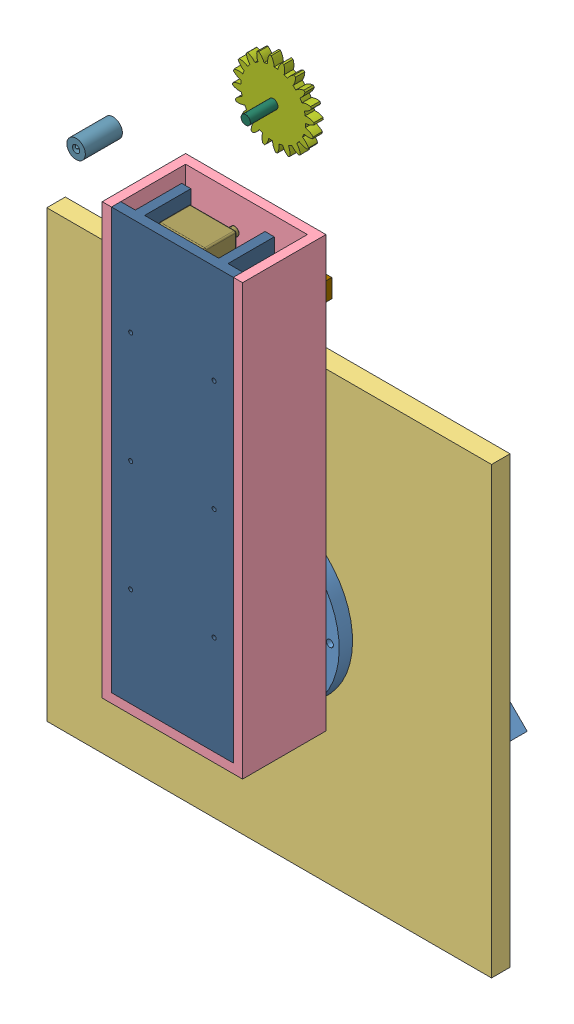
SolidWorks assembly Arm_Full_Assem, configuration Default. Lengths in mm.
Overall size (304.8 505.93 118.61).
59 component instances, 30 part files, 109 mates.
Components (placement in the parent):
- Bearing-1: Bearing [Default] at (11.5938 121.0098 145.145) x (0 1 0) z (0 0 1) size (114.3 114.3 9.17)
  - Outside_Ring-1: Outside_Ring [Default] at (-40.6964 23.8939 0.6571) size (114.3 114.3 9.17)
  - Inside_Ring-1: Inside_Ring [Default] at (-40.6964 23.8939 0.6571) size (92.08 92.08 9.17)
- Dummy_Backplate-1: Dummy_Backplate [Default] at (-12.3001 80.3134 133.1021) size (304.8 304.8 12.7)
- Bottom_Channel-1: Bottom_Channel [Default] at (-12.3001 26.9734 161.3215) x (-1 0 0) z (0 1 0) size (96.2 57.15 294.64)
- Pancake_Motor-1: Pancake_Motor [Default] at (-16.7001 240.6134 172.9215) x (-1 0 0) z (0 0 -1) size (42 42 23.6)
- rack spur rectangular_ai-2: rack spur rectangular_ai [Inch - Rack-spur - rectangular 40DP 20PA .25FW .125PH 9L---SAll] at (-37.7001 33.3234 173.9215) x (0 1 0) z (0 0 -1) size (228.6 3.81 6.35)
- spur gear_ai-7: spur gear_ai [Inch - Spur gear 40DP 56T 20PA .25FW ---S56N3.0H2.0L0.25N] at (-16.7001 240.6134 172.9215) x (0 0 1) z (-0.36764 0.929968 0) size (6.35 36.79 36.79)
- rack spur rectangular_ai-5: rack spur rectangular_ai [Inch - Rack-spur - rectangular 40DP 20PA .25FW .125PH 9L---SAll] at (13.0999 33.3234 180.2715) x (0 1 0) z (0 0 1) size (228.6 3.81 6.35)
- Motor_Gear-9: Motor_Gear [Default] at (-7.8101 206.1826 179.2715) x (-0.152038 -0.988375 0) z (0 0 -1) size (36.82 36.82 6.35)
- Bearing_Holder-1: Bearing_Holder [Default] at (-7.8101 195.1844 161.3215) x (0 -1 0) z (-1 0 0) size (24.67 10.16 41.05)
- Inside_Channel-1: Inside_Channel [Default] at (-44.0501 321.6134 174.0215) x (1 0 0) z (0 -1 0) size (83.5 38.1 288.29)
- Pancake_Motor-2: Pancake_Motor [Default] at (-12.3001 300.6134 194.1715) size (42 42 23.6) (hidden)
- spur gear_ai-11: spur gear_ai [Inch - Spur gear 10DP 20T 20PA 0.25FW ---S20N3.0H2.0L0.25N] at (13.4139 394.7961 162.3121) x (0 0 1) z (0.75856 -0.651603 0) size (6.35 55.38 55.38)
- Idler_Gear-12: Idler_Gear [Default] at (-28.1751 160.3234 180.2715) x (-0.966658 -0.256072 0) z (0 0 -1) size (13.95 13.95 6.35)
- Idler_Gear-13: Idler_Gear [Default] at (3.5749 160.3234 180.2715) x (-0.835792 0.549046 0) z (0 0 -1) size (13.95 13.95 6.35)
- Slip_Ring-1: Slip_Ring [Default] at (-12.3001 80.3134 121.1771) x (-0.506377 -0.862312 0) z (0 0 1) size (44 44 39.4)
- spur gear_ai-15: spur gear_ai [Inch - Spur gear 10DP 40T 20PA .25FW ---S40N3.0H2.0L0.25N] at (59.542 8.4713 129.9271) x (0 0 -1) z (0.885459 0.464717 0) size (6.35 106.46 106.46)
- Encoder-1: Encoder [Default] at (45.4422 5.6005 93.5071) x (0.707107 -0.707107 0) z (0 0 1) size (15.88 21.21 36.42)
- spur gear_ai-16: spur gear_ai [Inch - Spur gear 10DP 40T 20PA .25FW ---S40N3.0H2.0L0.5N] at (-84.1421 152.1554 129.9271) x (0 0 -1) z (-0.884026 -0.467439 0) size (6.35 106.46 106.46)
- Coupling-1: Coupling [Default] at (-90.1246 332.1277 174.8996) x (0.44043 -0.897787 0) z (0 0 1) size (12.7 12.7 25.4)
- Gear_Shaft-1: Gear_Shaft [Default] at (13.4139 394.7961 187.5996) x (-0.201369 0.979515 0) z (0 0 -1) size (6.35 6.35 19.05)
- Center_Gear-1: Center_Gear [Default] at (-12.3001 80.3134 123.5771) x (-0.493596 0.869691 0) z (0 0 1) size (106.51 106.51 6.35)
- Small_Bearing_Holder-1: Small_Bearing_Holder [Default] at (-44.8751 160.3234 161.3215) x (-1 0 0) z (0 0 -1) size (19.05 33.4 7.3)
- Small_Bearing_Holder-2: Small_Bearing_Holder [Default] at (-13.1251 160.3234 161.3215) x (-1 0 0) z (0 0 -1) size (19.05 33.4 7.3)
- 10mm_Bearing-2: 10mm_Bearing [7804K1] at (3.5749 160.3234 163.3215) x (0.99661 0.082273 0) z (0 0 1) size (10 10 4)
- Encoder_Holder-1: Encoder_Holder [Default] at (0.1843 -23.9456 104.5271) x (0.707107 0.707107 0) z (0 0 -1) size (152.4 38.1 34.92)
- 5_16_Bearing-3: 5_16_Bearing [60355K503] at (-84.1421 152.1554 140.2459) x (-0.2744 -0.961616 0) z (0 0 1) size (15.88 15.88 4.76)
- 5_16_Bearing-5: 5_16_Bearing [60355K503] at (59.542 8.4713 140.2459) size (15.88 15.88 4.76)
- Track2-1: Track2 [6723K25] at (-54.0501 158.3234 189.8965) x (0 0 -1) z (0 -1 0) size (27 8.7 250)
- Carriage2-1: Carriage2 [6723K11] at (-53.9501 53.3234 189.9465) x (0 0 -1) z (0 -1 0) size (23.9 5.35 40)
- Carriage2-2: Carriage2 [6723K11] at (29.3499 53.3234 189.9465) x (0 0 -1) z (0 1 0) size (23.9 5.35 40)
- Track2-2: Track2 [6723K25] at (29.4499 158.3234 189.8965) x (0 0 -1) z (0 1 0) size (27 8.7 250)
- Copper_Insert-1: Copper_Insert [Default] at (13.0999 258.1134 167.6715) x (1 0 0) z (0 -1 0) size (6.35 6.35 224.79)
- Rubber_Insulator-1: Rubber_Insulator [Default] at (19.4499 258.1134 161.3215) x (1 0 0) z (0 -1 0) size (3.17 12.7 224.79)
- Copper_Insert-2: Copper_Insert [Default] at (22.6249 258.1134 167.6715) x (1 0 0) z (0 -1 0) size (6.35 6.35 224.79)
- Copper_Insert-3: Copper_Insert [Default] at (-47.2251 33.3234 167.6715) x (-1 0 0) z (0 1 0) size (6.35 6.35 224.79)
- Rubber_Insulator-2: Rubber_Insulator [Default] at (-44.0501 33.3234 161.3215) x (-1 0 0) z (0 1 0) size (3.17 12.7 224.79)
- Copper_Insert-5: Copper_Insert [Default] at (-37.7001 33.3234 167.6715) x (-1 0 0) z (0 1 0) size (6.35 6.35 224.79)
- Graphite_Brush-1: Graphite_Brush [Default] at (22.568 289.9752 170.3294) x (1 0 0) z (0 0 -1) size (5.52 5.52 23.23)
  - Graphite-1: Graphite [Default] at (0.6919 3.2868 2.6579) size (5.08 5.08 10.16)
  - Graphite_Spring-1: Graphite_Spring [9657K268] at (3.2319 5.8268 25.5179) size (5.52 5.52 13.07)
- Graphite_Brush-2: Graphite_Brush [Default] at (13.043 289.9752 170.3294) x (1 0 0) z (0 0 -1) size (5.52 5.52 23.23)
  - Graphite-1: Graphite [Default] at (0.6919 3.2868 2.6579) size (5.08 5.08 10.16)
  - Graphite_Spring-1: Graphite_Spring [9657K268] at (3.2319 5.8268 25.5179) size (5.52 5.52 13.07)
- Graphite_Brush-3: Graphite_Brush [Default] at (-37.6431 278.3216 170.3294) x (-1 0 0) z (0 0 -1) size (5.52 5.52 23.23)
  - Graphite-1: Graphite [Default] at (0.6919 3.2868 2.6579) size (5.08 5.08 10.16)
  - Graphite_Spring-1: Graphite_Spring [9657K268] at (3.2319 5.8268 25.5179) size (5.52 5.52 13.07)
- Graphite_Brush-4: Graphite_Brush [Default] at (-47.1681 278.3216 170.3294) x (-1 0 0) z (0 0 -1) size (5.52 5.52 23.23)
  - Graphite-1: Graphite [Default] at (0.6919 3.2868 2.6579) size (5.08 5.08 10.16)
  - Graphite_Spring-1: Graphite_Spring [9657K268] at (3.2319 5.8268 25.5179) size (5.52 5.52 13.07)
- Brush_Holder-1: Brush_Holder [Default] at (9.9249 284.1484 147.3515) x (0 1 0) z (1 0 0) size (25.4 7.62 22.23)
- Brush_Holder-2: Brush_Holder [Default] at (-56.7501 284.1484 147.3515) x (0 1 0) z (1 0 0) size (25.4 7.62 22.23)
- Small_Gear_Shaft-1: Small_Gear_Shaft [Default] at (-28.1751 160.3234 166.2715) x (-0.966658 -0.256072 0) z (0 0 1) size (6.35 6.35 14)
- Small_Gear_Shaft-2: Small_Gear_Shaft [Default] at (3.5749 160.3234 166.2715) x (-0.835792 0.549046 0) z (0 0 1) size (6.35 6.35 14)
- Small_Gear_Shaft-3: Small_Gear_Shaft [Large_Gear] at (-7.8101 206.1826 165.2715) x (0.152038 0.988375 0) z (0 0 1) size (10 10 10.95)
- 10mm_Bearing-3: 10mm_Bearing [7804K1] at (-28.1751 160.3234 163.3215) x (0.999767 0.021604 0) z (0 0 1) size (10 10 4)
- 22mm_Bearing-1: 22mm_Bearing [5972K91] at (-7.8101 206.1826 164.8215) x (0.980177 0.198125 0) z (0 0 1) size (22 22 7)
- 1P0000_BrushMotor-1: 1P0000_BrushMotor [Default] at (-28.3001 276.3134 184.2715) x (0 1 0) z (-1 0 0) size (80 40 32)
Mates (geometry in assembly coordinates):
- Coincident1: coincident: plane of Bearing-1/Outside_Ring-1 through (-12.3001 80.3134 145.8021) normal (0 0 -1); plane of Dummy_Backplate-1 through (-12.3001 80.3134 145.8021) normal (0 0 1)
- Concentric1: concentric: circle of Bearing-1/Inside_Ring-1; circle of Dummy_Backplate-1
- Concentric2: concentric: circle of Bearing-1/Inside_Ring-1; circle of Bottom_Channel-1
- Concentric3: concentric: circle of Bearing-1/Inside_Ring-1; circle of Bottom_Channel-1
- Coincident4: coincident: plane of Bearing-1/Inside_Ring-1 through (-12.3001 80.3134 154.9715) normal (0 0 1); plane of Bottom_Channel-1 through (-60.4001 321.6134 154.9715) normal (0 0 -1)
- Coincident5: coincident: plane of Bottom_Channel-1 through (-12.3001 321.6134 161.3215) normal (0 0 1); plane of Pancake_Motor-1 through (-16.7001 240.6134 161.3215) normal (0 0 -1)
- Distance1: distance = 60 mm: plane of Pancake_Motor-1 through (-37.7001 261.6134 161.3215) normal (0 1 0); plane of Bottom_Channel-1 through (-12.3001 321.6134 161.3215) normal (0 1 0)
- Distance6: distance = 16.35 mm: plane of Bottom_Channel-1 through (-54.0501 321.6134 183.5465) normal (1 0 0); plane of Pancake_Motor-1 through (-37.7001 261.6134 161.3215) normal (-1 0 0)
- Distance3: distance = 1 mm: plane of rack spur rectangular_ai-2 through (-33.8901 33.3234 173.9215) normal (0 0 -1); plane of Pancake_Motor-1 through (-16.7001 240.6134 172.9215) normal (0 0 1)
- Coincident13: coincident: plane of Pancake_Motor-1 through (-16.7001 240.6134 172.9215) normal (0 0 1); plane of spur gear_ai-7 through (-16.7001 240.6134 172.9215) normal (0 0 -1)
- Concentric6: concentric: circle of Pancake_Motor-1; cylinder of spur gear_ai-7 through (-16.7001 240.6134 223.7216) axis (0 0 -1) radius 3.175
- Coincident54: coincident: plane of rack spur rectangular_ai-5 through (13.0999 33.3234 173.9215) normal (1 0 0); plane of Inside_Channel-1 through (13.0999 33.3234 174.0215) normal (-1 0 0)
- Distance11: distance = 1 mm: plane of Pancake_Motor-1 through (-16.7001 240.6134 172.9215) normal (0 0 1); plane of rack spur rectangular_ai-5 through (9.2899 33.3234 173.9215) normal (0 0 -1)
- Coincident17: coincident: plane of rack spur rectangular_ai-2 through (-37.7001 261.9234 180.2715) normal (0 1 0); plane of rack spur rectangular_ai-5 through (13.0999 261.9234 173.9215) normal (0 1 0)
- Concentric8: concentric: circle of Bottom_Channel-1; circle of Bearing_Holder-1
- Coincident20: coincident: plane of Bottom_Channel-1 through (-12.3001 321.6134 161.3215) normal (0 0 1); plane of Bearing_Holder-1 through (-7.8101 195.1844 161.3215) normal (0 0 -1)
- RackPinionMate1: rack pinion = 35.56 mm: line of rack spur rectangular_ai-2 through (-37.7001 33.3234 180.2715) axis (0 1 0); circle of spur gear_ai-7
- Distance16: distance = 10 mm: plane of Bottom_Channel-1 through (29.4499 321.6134 183.5465) normal (-1 0 0); plane of Inside_Channel-1 through (19.4499 33.3234 183.5465) normal (1 0 0)
- Coincident23: coincident: plane of rack spur rectangular_ai-5 through (13.0999 33.3234 173.9215) normal (0 -1 0); plane of Inside_Channel-1 through (-44.0501 33.3234 174.0215) normal (0 -1 0)
- LimitDistance1: limit distance = 0 mm: plane of Inside_Channel-1 through (-44.0501 33.3234 174.0215) normal (0 -1 0); plane of Bottom_Channel-1 through (-54.0501 33.3234 295.8626) normal (0 1 0)
- Coincident24: coincident: plane of Inside_Channel-1 through (-37.7001 33.3234 205.7715) normal (0 0 -1); plane of Pancake_Motor-2 through (-12.3001 300.6134 205.7715) normal (0 0 1)
- Width1: width: plane of Bottom_Channel-1 through (29.4499 321.6134 183.5465) normal (-1 0 0); plane of Bottom_Channel-1 through (-54.0501 321.6134 183.5465) normal (1 0 0); plane of Pancake_Motor-2 through (8.6999 321.6134 205.7715) normal (1 0 0); plane of Pancake_Motor-2 through (-33.3001 321.6134 205.7715) normal (-1 0 0)
- Coincident25: coincident: line of Inside_Channel-1 through (-37.7001 321.6134 205.7715) axis (1 0 0); line of Pancake_Motor-2 through (8.6999 321.6134 205.7715) axis (-1 0 0)
- Concentric9: concentric: circle of Pancake_Motor-2; circle of spur gear_ai-11
- Distance8: distance = 22.86 mm: plane of spur gear_ai-11 through (13.4139 394.7961 168.6621) normal (0 0 1); plane of Dummy_Backplate-1 through (-12.3001 80.3134 145.8021) normal (0 0 1)
- Parallel1: parallel: plane of Bottom_Channel-1 through (35.7999 321.6134 212.1215) normal (1 0 0); plane of assembly through (0 0 0) normal (1 0 0)
- Distance13: distance = 3.175 mm: plane of spur gear_ai-15 through (59.542 8.4713 129.9271) normal (0 0 1); plane of Dummy_Backplate-1 through (-12.3001 80.3134 133.1021) normal (0 0 -1)
- Concentric14: concentric: circle of spur gear_ai-15; circle of Encoder-1
- Coincident30: coincident: plane of spur gear_ai-15 through (59.542 8.4713 129.9271) normal (0 0 1); plane of Encoder-1 through (45.4422 5.6005 129.9271) normal (0 0 1)
- Concentric15: concentric: circle of spur gear_ai-15; circle of Dummy_Backplate-1
- Concentric16: concentric: circle of spur gear_ai-16; cylinder of Dummy_Backplate-1 through (-84.1421 152.1554 168.2527) axis (0 0 -1) radius 7.9375
- Distance14: distance = 3.175 mm: plane of spur gear_ai-16 through (-84.1421 152.1554 129.9271) normal (0 0 1); plane of Dummy_Backplate-1 through (-12.3001 80.3134 133.1021) normal (0 0 -1)
- Concentric17: concentric: circle of Pancake_Motor-2; circle of Coupling-1
- Coincident32: coincident: plane of Pancake_Motor-2 through (-12.3001 300.6134 194.1715) normal (0 0 -1); plane of Coupling-1 through (-12.3001 300.6134 194.1715) normal (0 0 1)
- Concentric18: concentric: circle of spur gear_ai-11; circle of Gear_Shaft-1
- Coincident34: coincident: plane of Coupling-1 through (-90.1246 332.1277 187.5996) normal (0 0 -1); plane of Gear_Shaft-1 through (13.4139 394.7961 187.5996) normal (0 0 1)
- Distance15: distance = 3.175 mm: plane of Center_Gear-1 through (-10.6229 56.5042 129.9271) normal (0 0 1); plane of Dummy_Backplate-1 through (-12.3001 80.3134 133.1021) normal (0 0 -1)
- Concentric19: concentric: circle of Bearing-1/Outside_Ring-1; circle of Center_Gear-1
- Concentric20: concentric: circle of Bearing-1/Inside_Ring-1; circle of Center_Gear-1
- Concentric21: concentric: circle of Slip_Ring-1; circle of Center_Gear-1
- Concentric22: concentric: circle of Slip_Ring-1; circle of Center_Gear-1
- Coincident39: coincident: plane of Slip_Ring-1 through (-12.3001 80.3134 123.5771) normal (0 0 1); plane of Center_Gear-1 through (-10.6229 56.5042 123.5771) normal (0 0 -1)
- GearMate2: gear = 60.3225 : 95.2475 mm: circle of Center_Gear-1; circle of spur gear_ai-15
- GearMate3: gear = 95.2475 : 60.3225 mm: circle of spur gear_ai-16; circle of Center_Gear-1
- Coincident40: coincident: plane of Bottom_Channel-1 through (-54.0501 321.6134 212.1215) normal (0 0 1); plane of Inside_Channel-1 through (-44.0501 33.3234 212.1215) normal (0 0 1)
- Parallel2: parallel: plane of Pancake_Motor-1 through (-37.7001 219.6134 161.3215) normal (0 -1 0); plane of Bearing_Holder-1 through (9.3584 218.4508 124.7233) normal (0 1 0)
- Coincident43: coincident: plane of Bottom_Channel-1 through (-12.3001 321.6134 161.3215) normal (0 0 1); plane of Small_Bearing_Holder-1 through (-44.8751 160.3234 161.3215) normal (0 0 -1)
- Parallel3: parallel: plane of Bottom_Channel-1 through (-54.0501 321.6134 183.5465) normal (1 0 0); plane of Small_Bearing_Holder-1 through (-18.6501 144.4484 120.6617) normal (1 0 0)
- Coincident45: coincident: plane of Bottom_Channel-1 through (-12.3001 321.6134 161.3215) normal (0 0 1); plane of Small_Bearing_Holder-2 through (-13.1251 160.3234 161.3215) normal (0 0 -1)
- Concentric25: concentric: cylinder of Bottom_Channel-1 through (3.5749 160.3234 212.1215) axis (0 0 -1) radius 3.175; circle of Small_Bearing_Holder-2
- Parallel4: parallel: plane of Bottom_Channel-1 through (29.4499 321.6134 183.5465) normal (-1 0 0); plane of Small_Bearing_Holder-2 through (-5.9501 144.4484 120.6617) normal (-1 0 0)
- Concentric26: concentric: circle of Small_Bearing_Holder-2; circle of 10mm_Bearing-2
- Coincident47: coincident: plane of Bottom_Channel-1 through (-12.3001 321.6134 161.3215) normal (0 0 1); plane of 10mm_Bearing-2 through (3.18 165.1071 161.3215) normal (0 0 -1)
- Coincident48: coincident: plane of Dummy_Backplate-1 through (-12.3001 80.3134 133.1021) normal (0 0 -1); plane of Encoder_Holder-1 through (0.1843 -23.9456 133.1021) normal (0 0 1)
- Coincident49: coincident: plane of Encoder-1 through (45.4422 5.6005 107.3971) normal (-0.707107 0.707107 0); plane of Encoder_Holder-1 through (45.443 5.6012 98.1771) normal (0.707107 -0.707107 0)
- Coincident50: coincident: plane of Encoder-1 through (60.44 20.5982 107.3971) normal (0.707107 0.707107 0); plane of Encoder_Holder-1 through (60.44 20.5982 98.1771) normal (-0.707107 -0.707107 0)
- Angle1: planar angle = 0.785398 rad: plane of Dummy_Backplate-1 through (140.0999 -72.0866 145.8021) normal (0 -1 0); plane of Encoder_Holder-1 through (27.125 -50.8864 98.1771) normal (0.707107 -0.707107 0)
- Concentric27: concentric: circle of Dummy_Backplate-1; circle of 5_16_Bearing-3
- Coincident51: coincident: plane of Dummy_Backplate-1 through (-12.3001 80.3134 142.6271) normal (0 0 -1); plane of 5_16_Bearing-3 through (-76.7383 150.0427 142.6271) normal (0 0 1)
- Concentric28: concentric: circle of Dummy_Backplate-1; circle of 5_16_Bearing-5
- Coincident53: coincident: plane of Dummy_Backplate-1 through (-12.3001 80.3134 142.6271) normal (0 0 -1); plane of 5_16_Bearing-5 through (59.542 16.1707 142.6271) normal (0 0 1)
- Coincident56: coincident: plane of rack spur rectangular_ai-2 through (-37.7001 33.3234 180.2715) normal (-1 0 0); plane of Inside_Channel-1 through (-37.7001 33.3234 174.0215) normal (1 0 0)
- Coincident65: coincident: plane of Bottom_Channel-1 through (-54.0501 321.6134 183.5465) normal (1 0 0); plane of Track2-1 through (-54.0501 33.3234 200.8965) normal (-1 0 0)
- Coincident66: coincident: plane of Bottom_Channel-1 through (-54.0501 33.3234 295.8626) normal (0 1 0); plane of Track2-1 through (-52.7501 33.3234 200.6965) normal (0 -1 0)
- Width2: width: plane of Inside_Channel-1 through (-44.0501 33.3234 205.7715) normal (0 0 -1); plane of Inside_Channel-1 through (-44.0501 33.3234 174.0215) normal (0 0 -1); plane of Track2-1 through (-50.0501 33.3234 176.3965) normal (0 0 -1); plane of Track2-1 through (-46.3501 33.3234 203.3965) normal (0 0 1)
- Coincident67: coincident: plane of Track2-1 through (-49.4501 33.3234 201.8965) normal (0 0 -1); plane of Carriage2-1 through (-47.0271 33.3234 201.8965) normal (0 0 1)
- Coincident69: coincident: plane of Inside_Channel-1 through (-44.0501 33.3234 174.0215) normal (0 -1 0); plane of Carriage2-1 through (-48.1501 33.3234 189.9465) normal (0 -1 0)
- Coincident71: coincident: plane of Track2-1 through (-46.4501 33.3234 181.1465) normal (-1 0 0); plane of Carriage2-1 through (-46.4501 33.3234 178.5735) normal (1 0 0)
- Coincident72: coincident: plane of Inside_Channel-1 through (13.0999 33.3234 174.0215) normal (0 0 -1); plane of Copper_Insert-1 through (13.0999 33.3234 174.0215) normal (0 0 1)
- Coincident82: coincident: plane of Inside_Channel-1 through (13.0999 33.3234 174.0215) normal (-1 0 0); plane of Copper_Insert-1 through (13.0999 33.3234 167.6715) normal (-1 0 0)
- Distance18: distance = 63.5 mm: plane of Inside_Channel-1 through (-44.0501 321.6134 174.0215) normal (0 1 0); plane of Copper_Insert-1 through (13.0999 258.1134 167.6715) normal (0 1 0)
- Coincident74: coincident: plane of Copper_Insert-1 through (19.4499 33.3234 167.6715) normal (1 0 0); plane of Rubber_Insulator-1 through (19.4499 33.3234 161.3215) normal (-1 0 0)
- Coincident75: coincident: plane of Copper_Insert-1 through (13.0999 258.1134 167.6715) normal (0 1 0); plane of Rubber_Insulator-1 through (19.4499 258.1134 161.3215) normal (0 1 0)
- Coincident76: coincident: plane of Inside_Channel-1 through (13.0999 33.3234 174.0215) normal (0 0 -1); plane of Rubber_Insulator-1 through (19.4499 33.3234 174.0215) normal (0 0 1)
- Coincident78: coincident: plane of Copper_Insert-1 through (13.0999 258.1134 167.6715) normal (0 1 0); plane of Copper_Insert-2 through (22.6249 258.1134 167.6715) normal (0 1 0)
- Coincident79: coincident: plane of Rubber_Insulator-1 through (22.6249 33.3234 161.3215) normal (1 0 0); plane of Copper_Insert-2 through (22.6249 33.3234 167.6715) normal (-1 0 0)
- Coincident80: coincident: plane of Copper_Insert-1 through (13.0999 33.3234 167.6715) normal (0 0 -1); plane of Copper_Insert-2 through (22.6249 33.3234 167.6715) normal (0 0 -1)
- Width3: width: plane of Bottom_Channel-1 through (22.6249 287.3234 145.9913) normal (1 0 0); plane of Bottom_Channel-1 through (28.9749 287.3234 145.9913) normal (-1 0 0); plane of Graphite_Brush-1/Graphite-1 through (28.3399 286.6884 157.5115) normal (1 0 0); plane of Graphite_Brush-1/Graphite-1 through (23.2599 286.6884 157.5115) normal (-1 0 0)
- Width4: width: plane of Bottom_Channel-1 through (28.9749 287.3234 145.9913) normal (-1 0 0); plane of Bottom_Channel-1 through (22.6249 287.3234 145.9913) normal (1 0 0); plane of Graphite_Brush-1/Graphite-1 through (28.3399 286.6884 157.5115) normal (1 0 0); plane of Graphite_Brush-1/Graphite-1 through (23.2599 286.6884 157.5115) normal (-1 0 0)
- Width5: width: plane of Bottom_Channel-1 through (22.6249 280.9734 145.9913) normal (0 1 0); plane of Bottom_Channel-1 through (22.6249 287.3234 145.9913) normal (0 -1 0); plane of Graphite_Brush-1/Graphite-1 through (23.2599 286.6884 157.5115) normal (0 1 0); plane of Graphite_Brush-1/Graphite-1 through (23.2599 281.6084 157.5115) normal (0 -1 0)
- Coincident83: coincident: plane of Copper_Insert-2 through (22.6249 33.3234 167.6715) normal (0 0 -1); plane of Graphite_Brush-1/Graphite-1 through (23.2599 286.6884 167.6715) normal (0 0 1)
- Coincident85: coincident: line of Bottom_Channel-1 through (28.9749 287.3234 154.9715) axis (-1 0 0); line of Brush_Holder-1 through (22.6249 287.3234 154.9715) axis (1 0 0)
- Coincident86: coincident: plane of Bottom_Channel-1 through (-60.4001 321.6134 154.9715) normal (0 0 -1); plane of Brush_Holder-1 through (21.0374 284.1484 154.9715) normal (0 0 1)
- Coincident87: coincident: line of Bottom_Channel-1 through (28.9749 280.9734 154.9715) axis (0 1 0); line of Brush_Holder-1 through (28.9749 287.3234 154.9715) axis (0 -1 0)
- Concentric32: concentric: circle of Small_Bearing_Holder-1; circle of 10mm_Bearing-3
- Coincident94: coincident: plane of Bottom_Channel-1 through (-12.3001 321.6134 161.3215) normal (0 0 1); plane of 10mm_Bearing-3 through (-28.2788 165.1223 161.3215) normal (0 0 -1)
- Concentric33: concentric: circle of Bottom_Channel-1; circle of Small_Bearing_Holder-1
- Concentric34: concentric: circle of Bottom_Channel-1; circle of 22mm_Bearing-1
- Coincident95: coincident: plane of Bottom_Channel-1 through (-12.3001 321.6134 161.3215) normal (0 0 1); plane of 22mm_Bearing-1 through (-9.9201 216.6214 161.3215) normal (0 0 -1)
- Concentric35: concentric: circle of Motor_Gear-9; circle of 22mm_Bearing-1
- Coincident97: coincident: plane of Motor_Gear-9 through (-7.8101 206.1826 179.2715) normal (0 0 1); plane of Small_Gear_Shaft-3 through (-7.8101 206.1826 179.2715) normal (0 0 1)
- Coincident99: coincident: plane of Motor_Gear-9 through (-7.8101 206.1826 179.2715) normal (0 0 1); plane of spur gear_ai-7 through (-16.7001 240.6134 179.2715) normal (0 0 1)
- Concentric36: concentric: unknown of Motor_Gear-9; unknown of Small_Gear_Shaft-3
- GearMate4: gear = 33.9344 : 33.9344 mm: circle of Motor_Gear-9; circle of spur gear_ai-7
- Coincident100: coincident: line of Motor_Gear-9 through (-5.5892 203.9135 179.2715) axis (-0.988375 0.152038 0); line of Small_Gear_Shaft-3 through (-5.5892 203.9135 179.2715) axis (-0.988375 0.152038 0)
- Concentric37: concentric: circle of Idler_Gear-12; circle of Small_Gear_Shaft-1
- Concentric38: concentric: circle of Small_Gear_Shaft-1; circle of 10mm_Bearing-3
- Coincident102: coincident: plane of Idler_Gear-12 through (-31.1555 160.1863 180.2715) normal (0 0 1); plane of Small_Gear_Shaft-1 through (-28.1751 160.3234 180.2715) normal (0 0 1)
- Coincident103: coincident: plane of rack spur rectangular_ai-2 through (-33.8901 33.3234 180.2715) normal (0 0 1); plane of Idler_Gear-12 through (-31.1555 160.1863 180.2715) normal (0 0 1)
- Coincident104: coincident: line of Idler_Gear-12 through (-26.984 163.2665 180.2715) axis (0.256072 -0.966658 0); line of Small_Gear_Shaft-1 through (-26.984 163.2665 180.2715) axis (0.256072 -0.966658 0)
- RackPinionMate3: rack pinion = 11.0744 mm: line of rack spur rectangular_ai-2 through (-37.7001 33.3234 180.2715) axis (0 1 0); circle of Idler_Gear-12
- Concentric39: concentric: circle of 10mm_Bearing-2; circle of Small_Gear_Shaft-2
- Concentric40: concentric: circle of Idler_Gear-13; circle of Small_Gear_Shaft-2
- Coincident107: coincident: plane of Idler_Gear-13 through (1.4839 162.4516 180.2715) normal (0 0 1); plane of Small_Gear_Shaft-2 through (3.5749 160.3234 180.2715) normal (0 0 1)
- Coincident108: coincident: plane of rack spur rectangular_ai-5 through (9.2899 33.3234 180.2715) normal (0 0 1); plane of Idler_Gear-13 through (1.4839 162.4516 180.2715) normal (0 0 1)
- Coincident109: coincident: line of Idler_Gear-13 through (6.5617 161.4004 180.2715) axis (-0.549046 -0.835792 0); line of Small_Gear_Shaft-2 through (6.5617 161.4004 180.2715) axis (-0.549046 -0.835792 0)
- RackPinionMate4: rack pinion = 11.0744 mm: line of rack spur rectangular_ai-5 through (13.0999 33.3234 180.2715) axis (0 1 0); circle of Idler_Gear-13
- Coincident111: coincident: plane of Inside_Channel-1 through (-37.7001 33.3234 205.7715) normal (0 0 -1); plane of 1P0000_BrushMotor-1 through (-28.3001 276.3134 205.7715) normal (0 0 1)
- Coincident115: coincident: moEndPointRef_w of Inside_Channel-1; unknown of 1P0000_BrushMotor-1
